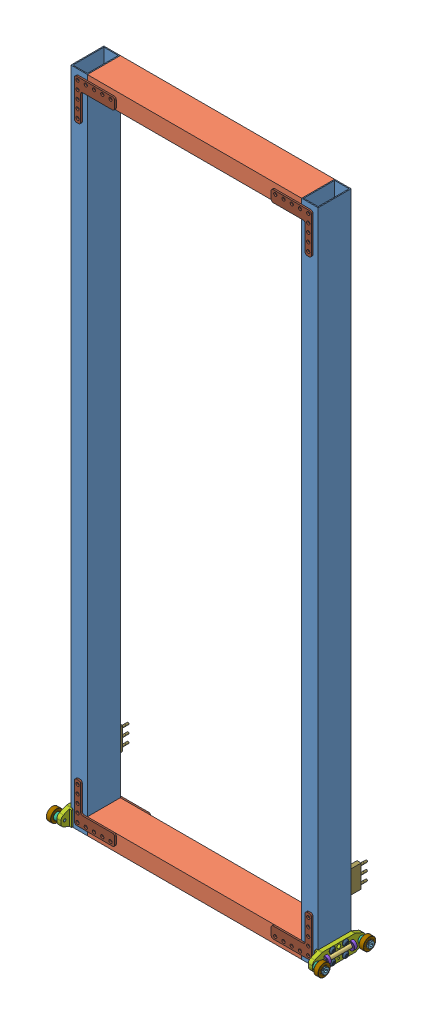
SolidWorks assembly Assem1^short elevator second stage(1), configuration Default. Lengths in mm.
Overall size (424.07 1018.01 128.54).
54 component instances, 12 part files, 44 mates.
Components (placement in the parent):
- 2x1 40in extrude-1: 2x1 40in extrude [Default] at (187.1883 1213.0001 1057.544) x (1 0 0) z (0 -1 0) size (25.4 50.8 1016)
- 2x1 40in extrude-2: 2x1 40in extrude [Default] at (542.7883 1213.0001 1057.544) x (1 0 0) z (0 -1 0) size (25.4 50.8 1016)
- 2x1 13in extrude-1: 2x1 13in extrude [Default] at (542.7883 197.0001 1108.344) x (0 0 1) z (0 -1 0) size (50.8 330.2 25.4)
- 2x1 13in extrude-2: 2x1 13in extrude [Default] at (542.7883 1187.6001 1108.344) x (0 0 1) z (0 -1 0) size (50.8 330.2 25.4)
- Bearing Block-1: Bearing Block [Default] at (-133.7189 -456.4617 -235.3019) x (-1 0 0) z (0 1 0) size (31.06 89.43 29.43)
  - Sliding Elevator Bearing Block Kit.step-1: Sliding Elevator Bearing Block Kit.step [Default] at (-2.279 1755.626 148.4607) x (0 -0.999847 -0.017493) z (-1 0 0) size (88.96 27.87 31.06)
    - .25diameter_1.75inSteelDowel_SLIDE-002.step-1: .25diameter_1.75inSteelDowel_SLIDE-002.step [Default] at (428.3334 525.2741 706.1052) x (0.999847 0.017493 0) z (0 0 1) size (44.45 6.35 6.35)
    - 10-32 Locknut 2623.step-1: 10-32 Locknut 2623.step [Default] at (418.0305 533.3501 696.4532) x (1 0 0) z (0 1 0) size (9.53 5.96 11)
    - Bearing Block Shoulder Bolt - SLIDE-004.step-1: Bearing Block Shoulder Bolt - SLIDE-004.step [Default] at (393.4137 524.6631 723.447) x (0.999978 0.006628 0) z (0 0 1) size (9.53 9.53 21.53)
    - Bearing Block Shoulder Bolt Spacer - SLIDE-003.step-1: Bearing Block Shoulder Bolt Spacer - SLIDE-003.step [Default] at (209.8469 202.8854 705.9782) x (0.999977 0.006804 0) z (0 0 1) size (10.72 10.72 5.56)
    - Sliding Bearing Block Plate - SLIDE-001.step-1: Sliding Bearing Block Plate - SLIDE-001.step [Default] at (417.8216 -325.94 699.6282) x (0.999847 0.017493 0) z (0 0 1) size (81.28 25.4 9.54)
    - TTB-0027_.50OD_.25ID_.188WD.step-1: TTB-0027_.50OD_.25ID_.188WD.step [Default] at (448.2757 525.623 706.1052) x (0 0 -1) z (0.999847 0.017493 0) size (12.7 12.7 4.76)
    - TTB-0038_75OD_25ID_28WD.step-1: TTB-0038_75OD_25ID_28WD.step [Default] at (463.253 525.885 715.1127) size (19.05 19.05 7.14)
    - Bearing Block Shoulder Bolt - SLIDE-004.step-2: Bearing Block Shoulder Bolt - SLIDE-004.step [Default] at (463.253 525.885 723.447) size (9.53 9.53 21.53)
    - TTB-0027_.50OD_.25ID_.188WD.step-2: TTB-0027_.50OD_.25ID_.188WD.step [Default] at (408.3911 524.9252 706.1052) x (0 0 -1) z (0.999847 0.017493 0) size (12.7 12.7 4.76)
    - Bearing Block Shoulder Bolt Spacer - SLIDE-003.step-2: Bearing Block Shoulder Bolt Spacer - SLIDE-003.step [Default] at (277.5012 205.3636 705.9782) size (10.72 10.72 5.56)
    - TTB-0038_75OD_25ID_28WD.step-2: TTB-0038_75OD_25ID_28WD.step [Default] at (393.4137 524.6631 715.1127) x (0.999973 0.007362 0) z (0 0 1) size (19.05 19.05 7.14)
    - .625 Long 10-32 Button Head Screw.step-1: .625 Long 10-32 Button Head Screw.step [Default] at (438.3474 533.7055 699.3234) x (0.999998 0.002032 0) z (0 0 1) size (9.17 9.17 18.44)
    - .625 Long 10-32 Button Head Screw.step-2: .625 Long 10-32 Button Head Screw.step [Default] at (438.6362 517.1981 699.3234) x (1 -0.000148 0) z (0 0 1) size (9.17 9.17 18.44)
    - .625 Long 10-32 Button Head Screw.step-3: .625 Long 10-32 Button Head Screw.step [Default] at (418.3193 516.8426 699.3234) x (0.999999 0.001159 0) z (0 0 1) size (9.17 9.17 18.44)
    - .625 Long 10-32 Button Head Screw.step-4: .625 Long 10-32 Button Head Screw.step [Default] at (418.0305 533.3501 699.3234) x (0.999983 0.005862 0) z (0 0 1) size (9.17 9.17 18.44)
    - 10-32 Locknut 2623.step-2: 10-32 Locknut 2623.step [Default] at (438.3474 533.7055 696.4532) x (0.999999 0.001134 0) z (-0.001134 0.999999 0) size (9.53 5.96 11)
    - 10-32 Locknut 2623.step-3: 10-32 Locknut 2623.step [Default] at (438.6362 517.1981 696.4532) x (1 0.000493 0) z (-0.000493 1 0) size (9.53 5.96 11)
    - 10-32 Locknut 2623.step-4: 10-32 Locknut 2623.step [Default] at (418.3193 516.8426 696.4532) x (0.999999 0.001452 0) z (-0.001452 0.999999 0) size (9.53 5.96 11)
- Copy of Copy (4) of Assem10^Assem1_short elevator second stage(1)-1: Copy of Copy (4) of Assem10^Assem1_short elevator second stage(1) [Default] at (889.0955 875.8618 -235.1495) x (1 0 0) z (0 -1 0) size (31.06 89.43 29.43) (virtual)
  - Sliding Elevator Bearing Block Kit.step-1: Sliding Elevator Bearing Block Kit.step [Default] at (-2.279 1755.626 148.4607) x (0 -0.999847 -0.017493) z (-1 0 0) size (88.96 27.87 31.06)
    - .25diameter_1.75inSteelDowel_SLIDE-002.step-1: .25diameter_1.75inSteelDowel_SLIDE-002.step [Default] at (428.3334 525.2741 706.1052) x (0.999847 0.017493 0) z (0 0 1) size (44.45 6.35 6.35)
    - 10-32 Locknut 2623.step-1: 10-32 Locknut 2623.step [Default] at (418.0305 533.3501 696.4532) x (1 0 0) z (0 1 0) size (9.53 5.96 11)
    - Bearing Block Shoulder Bolt - SLIDE-004.step-1: Bearing Block Shoulder Bolt - SLIDE-004.step [Default] at (393.4137 524.6631 723.447) x (0.999978 0.006628 0) z (0 0 1) size (9.53 9.53 21.53)
    - Bearing Block Shoulder Bolt Spacer - SLIDE-003.step-1: Bearing Block Shoulder Bolt Spacer - SLIDE-003.step [Default] at (209.8469 202.8854 705.9782) x (0.999977 0.006804 0) z (0 0 1) size (10.72 10.72 5.56)
    - Sliding Bearing Block Plate - SLIDE-001.step-1: Sliding Bearing Block Plate - SLIDE-001.step [Default] at (417.8216 -325.94 699.6282) x (0.999847 0.017493 0) z (0 0 1) size (81.28 25.4 9.54)
    - TTB-0027_.50OD_.25ID_.188WD.step-1: TTB-0027_.50OD_.25ID_.188WD.step [Default] at (448.2757 525.623 706.1052) x (0 0 -1) z (0.999847 0.017493 0) size (12.7 12.7 4.76)
    - TTB-0038_75OD_25ID_28WD.step-1: TTB-0038_75OD_25ID_28WD.step [Default] at (463.253 525.885 715.1127) size (19.05 19.05 7.14)
    - Bearing Block Shoulder Bolt - SLIDE-004.step-2: Bearing Block Shoulder Bolt - SLIDE-004.step [Default] at (463.253 525.885 723.447) size (9.53 9.53 21.53)
    - TTB-0027_.50OD_.25ID_.188WD.step-2: TTB-0027_.50OD_.25ID_.188WD.step [Default] at (408.3911 524.9252 706.1052) x (0 0 -1) z (0.999847 0.017493 0) size (12.7 12.7 4.76)
    - Bearing Block Shoulder Bolt Spacer - SLIDE-003.step-2: Bearing Block Shoulder Bolt Spacer - SLIDE-003.step [Default] at (277.5012 205.3636 705.9782) size (10.72 10.72 5.56)
    - TTB-0038_75OD_25ID_28WD.step-2: TTB-0038_75OD_25ID_28WD.step [Default] at (393.4137 524.6631 715.1127) x (0.999973 0.007362 0) z (0 0 1) size (19.05 19.05 7.14)
    - .625 Long 10-32 Button Head Screw.step-1: .625 Long 10-32 Button Head Screw.step [Default] at (438.3474 533.7055 699.3234) x (0.999998 0.002032 0) z (0 0 1) size (9.17 9.17 18.44)
    - .625 Long 10-32 Button Head Screw.step-2: .625 Long 10-32 Button Head Screw.step [Default] at (438.6362 517.1981 699.3234) x (1 -0.000148 0) z (0 0 1) size (9.17 9.17 18.44)
    - .625 Long 10-32 Button Head Screw.step-3: .625 Long 10-32 Button Head Screw.step [Default] at (418.3193 516.8426 699.3234) x (0.999999 0.001159 0) z (0 0 1) size (9.17 9.17 18.44)
    - .625 Long 10-32 Button Head Screw.step-4: .625 Long 10-32 Button Head Screw.step [Default] at (418.0305 533.3501 699.3234) x (0.999983 0.005862 0) z (0 0 1) size (9.17 9.17 18.44)
    - 10-32 Locknut 2623.step-2: 10-32 Locknut 2623.step [Default] at (438.3474 533.7055 696.4532) x (0.999999 0.001134 0) z (-0.001134 0.999999 0) size (9.53 5.96 11)
    - 10-32 Locknut 2623.step-3: 10-32 Locknut 2623.step [Default] at (438.6362 517.1981 696.4532) x (1 0.000493 0) z (-0.000493 1 0) size (9.53 5.96 11)
    - 10-32 Locknut 2623.step-4: 10-32 Locknut 2623.step [Default] at (418.3193 516.8426 696.4532) x (0.999999 0.001452 0) z (-0.001452 0.999999 0) size (9.53 5.96 11)
- L bracket thin-1: L bracket thin [Default] at (31.2018 194.4353 779.4446) x (-1 0 0) z (0 0.754511 0.656287) size (61.93 42.53 48.36)
- L bracket thin-2: L bracket thin [Default] at (31.2018 194.4353 726.1446) x (-1 0 0) z (0 0.754511 0.656287) size (61.93 42.53 48.36)
- L bracket thin-3: L bracket thin [Default] at (724.1747 194.4353 1439.7435) x (1 0 0) z (0 0.754511 -0.656287) size (61.93 42.53 48.36)
- L bracket thin-4: L bracket thin [Default] at (724.1747 194.4353 1386.4435) x (1 0 0) z (0 0.754511 -0.656287) size (61.93 42.53 48.36)
- L bracket thin-5: L bracket thin [Default] at (724.1747 1215.5648 779.4446) x (1 0 0) z (0 -0.754511 0.656287) size (61.93 42.53 48.36)
- L bracket thin-6: L bracket thin [Default] at (31.2018 1215.5648 1386.4435) x (-1 0 0) z (0 -0.754511 -0.656287) size (61.93 42.53 48.36)
- L bracket thin-7: L bracket thin [Default] at (31.2018 1215.5648 1439.7435) x (-1 0 0) z (0 -0.754511 -0.656287) size (61.93 42.53 48.36)
- L bracket thin-8: L bracket thin [Default] at (724.1747 1215.5648 726.1446) x (1 0 0) z (0 -0.754511 0.656287) size (61.93 42.53 48.36)
- chain block-1: chain block [Default] at (725.1399 192.8478 1386.4435) x (1 0 0) z (0 0.754511 -0.656287) size (13.97 43.8 43.91)
- chain block-2: chain block [Default] at (30.2366 375.7773 1386.4435) x (-1 0 0) z (0 -0.754511 -0.656287) size (13.97 43.8 43.91)
Mates (geometry in assembly coordinates):
- Coincident9: coincident anti-aligned: plane of 2x1 40in extrude-1 through (212.5883 197.0001 1057.544) normal (1 0 0); plane of 2x1 13in extrude-1 through (212.5883 197.0001 1108.344) normal (-1 0 0)
- Coincident10: coincident aligned: line of 2x1 40in extrude-1 through (212.5883 197.0001 1057.544) axis (0 0 1); line of 2x1 13in extrude-1 through (212.5883 197.0001 1057.544) axis (0 0 1)
- Coincident11: coincident aligned: line of 2x1 40in extrude-1 through (212.5883 197.0001 1108.344) axis (0 1 0); line of 2x1 13in extrude-1 through (212.5883 197.0001 1108.344) axis (0 1 0)
- Coincident14: coincident anti-aligned: plane of 2x1 40in extrude-1 through (212.5883 197.0001 1057.544) normal (1 0 0); plane of 2x1 13in extrude-2 through (212.5883 1187.6001 1108.344) normal (-1 0 0)
- Coincident15: coincident aligned: plane of 2x1 40in extrude-1 through (187.1883 197.0001 1108.344) normal (0 0 1); plane of 2x1 13in extrude-2 through (212.5883 1213.0001 1108.344) normal (0 0 1)
- Coincident16: coincident aligned: plane of 2x1 40in extrude-1 through (187.1883 1213.0001 1057.544) normal (0 1 0); plane of 2x1 13in extrude-2 through (212.5883 1213.0001 1057.544) normal (0 1 0)
- Coincident27: coincident anti-aligned: plane of 2x1 40in extrude-1 through (187.1883 197.0001 1057.544) normal (0 0 -1); plane of Copy of Copy (4) of Assem10^Assem2_short elevator(1)-1/Sliding Elevator Bearing Block Kit.step-1/Sliding Bearing Block Plate - SLIDE-001.step-1 through (187.1883 197.0001 1057.544) normal (0 0 1)
- Coincident28: coincident anti-aligned: plane of 2x1 40in extrude-1 through (187.1883 197.0001 1057.544) normal (-1 0 0); plane of Copy of Copy (4) of Assem10^Assem2_short elevator(1)-1/Sliding Elevator Bearing Block Kit.step-1/Sliding Bearing Block Plate - SLIDE-001.step-1 through (187.1883 209.7001 1083.0202) normal (1 0 0)
- Coincident29: coincident aligned: plane of 2x1 40in extrude-1 through (187.1883 197.0001 1057.544) normal (0 -1 0); plane of Copy of Copy (4) of Assem10^Assem2_short elevator(1)-1/Sliding Elevator Bearing Block Kit.step-1/Sliding Bearing Block Plate - SLIDE-001.step-1 through (187.1883 197.0001 1057.6202) normal (0 -1 0)
- Distance4: distance = 7.874 mm aligned: plane of 2x1 40in extrude-1 through (212.5883 197.0001 1057.544) normal (1 0 0); plane of L bracket thin-3 through (204.7143 222.4001 1110.844) normal (1 0 0)
- Distance5: distance = 7.874 mm aligned: plane of L bracket thin-4 through (204.7143 222.4001 1057.544) normal (1 0 0); plane of 2x1 40in extrude-1 through (212.5883 197.0001 1057.544) normal (1 0 0)
- Distance8: distance = 7.874 mm aligned: plane of L bracket thin-8 through (204.7143 1187.6001 1055.044) normal (1 0 0); plane of 2x1 40in extrude-1 through (212.5883 197.0001 1057.544) normal (1 0 0)
- Distance10: distance = 7.874 mm aligned: plane of 2x1 40in extrude-1 through (212.5883 197.0001 1057.544) normal (1 0 0); plane of L bracket thin-5 through (204.7143 1187.6001 1108.344) normal (1 0 0)
- Coincident78: coincident anti-aligned: plane of 2x1 40in extrude-1 through (187.1883 197.0001 1057.544) normal (0 0 -1); plane of chain block-1 through (198.6818 284.3126 1057.544) normal (0 0 1)
- Coincident12: coincident anti-aligned: line of 2x1 40in extrude-2 through (542.7883 197.0001 1108.344) axis (0 0 -1); line of 2x1 13in extrude-1 through (542.7883 197.0001 1057.544) axis (0 0 1)
- Coincident13: coincident aligned: plane of 2x1 40in extrude-2 through (542.7883 197.0001 1108.344) normal (0 0 1); plane of 2x1 13in extrude-1 through (212.5883 222.4001 1108.344) normal (0 0 1)
- Coincident24: coincident anti-aligned: plane of 2x1 40in extrude-2 through (568.1883 197.0001 1057.544) normal (1 0 0); plane of Copy of Copy (3) of Assem10^Assem2_short elevator(1)-1/Sliding Elevator Bearing Block Kit.step-1/Sliding Bearing Block Plate - SLIDE-001.step-1 through (568.1883 209.7001 1082.8678) normal (-1 0 0)
- Coincident25: coincident aligned: plane of 2x1 40in extrude-2 through (542.7883 197.0001 1057.544) normal (0 -1 0); plane of Copy of Copy (3) of Assem10^Assem2_short elevator(1)-1/Sliding Elevator Bearing Block Kit.step-1/Sliding Bearing Block Plate - SLIDE-001.step-1 through (568.1883 197.0001 1108.2678) normal (0 -1 0)
- Coincident26: coincident anti-aligned: plane of 2x1 40in extrude-2 through (542.7883 197.0001 1108.344) normal (0 0 1); plane of Copy of Copy (3) of Assem10^Assem2_short elevator(1)-1/Sliding Elevator Bearing Block Kit.step-1/Sliding Bearing Block Plate - SLIDE-001.step-1 through (568.1883 197.0001 1108.344) normal (0 0 -1)
- Distance3: distance = 7.874 mm aligned: plane of 2x1 40in extrude-2 through (542.7883 197.0001 1057.544) normal (-1 0 0); plane of L bracket thin-1 through (550.6623 222.4001 1108.344) normal (-1 0 0)
- Distance6: distance = 7.874 mm aligned: plane of 2x1 40in extrude-2 through (542.7883 197.0001 1057.544) normal (-1 0 0); plane of L bracket thin-2 through (550.6623 222.4001 1055.044) normal (-1 0 0)
- Distance7: distance = 7.874 mm aligned: plane of 2x1 40in extrude-2 through (542.7883 197.0001 1057.544) normal (-1 0 0); plane of L bracket thin-6 through (550.6623 1187.6001 1057.544) normal (-1 0 0)
- Distance9: distance = 7.874 mm aligned: plane of L bracket thin-7 through (550.6623 1187.6001 1110.844) normal (-1 0 0); plane of 2x1 40in extrude-2 through (542.7883 197.0001 1057.544) normal (-1 0 0)
- Coincident83: coincident anti-aligned: plane of 2x1 40in extrude-2 through (542.7883 197.0001 1057.544) normal (0 0 -1); plane of chain block-2 through (556.6948 284.3126 1057.544) normal (0 0 1)
- Coincident45: coincident anti-aligned: plane of 2x1 13in extrude-1 through (212.5883 222.4001 1108.344) normal (0 0 1); plane of L bracket thin-1 through (529.2501 235.8875 1108.344) normal (0 0 -1)
- Coincident47: coincident aligned: plane of 2x1 13in extrude-1 through (212.5883 222.4001 1057.544) normal (0 1 0); plane of L bracket thin-1 through (498.2875 222.4001 1110.844) normal (0 1 0)
- Coincident50: coincident anti-aligned: plane of 2x1 13in extrude-1 through (212.5883 222.4001 1108.344) normal (0 0 1); plane of L bracket thin-3 through (226.1265 235.8875 1108.344) normal (0 0 -1)
- Coincident51: coincident aligned: plane of 2x1 13in extrude-1 through (212.5883 222.4001 1057.544) normal (0 1 0); plane of L bracket thin-3 through (257.0891 222.4001 1108.344) normal (0 1 0)
- Coincident53: coincident anti-aligned: plane of 2x1 13in extrude-1 through (212.5883 222.4001 1057.544) normal (0 0 -1); plane of L bracket thin-4 through (226.1265 235.8875 1057.544) normal (0 0 1)
- Coincident55: coincident aligned: plane of 2x1 13in extrude-1 through (212.5883 222.4001 1057.544) normal (0 1 0); plane of L bracket thin-4 through (257.0891 222.4001 1055.044) normal (0 1 0)
- Coincident57: coincident anti-aligned: plane of 2x1 13in extrude-1 through (212.5883 222.4001 1057.544) normal (0 0 -1); plane of L bracket thin-2 through (529.2501 235.8875 1057.544) normal (0 0 1)
- Coincident58: coincident aligned: plane of 2x1 13in extrude-1 through (212.5883 222.4001 1057.544) normal (0 1 0); plane of L bracket thin-2 through (498.2875 222.4001 1057.544) normal (0 1 0)
- Coincident60: coincident anti-aligned: plane of 2x1 13in extrude-2 through (212.5883 1213.0001 1057.544) normal (0 0 -1); plane of L bracket thin-6 through (529.2501 1174.1127 1057.544) normal (0 0 1)
- Coincident61: coincident aligned: plane of 2x1 13in extrude-2 through (212.5883 1187.6001 1057.544) normal (0 -1 0); plane of L bracket thin-6 through (498.2875 1187.6001 1055.044) normal (0 -1 0)
- Coincident63: coincident anti-aligned: plane of 2x1 13in extrude-2 through (212.5883 1213.0001 1057.544) normal (0 0 -1); plane of L bracket thin-8 through (226.1265 1174.1127 1057.544) normal (0 0 1)
- Coincident64: coincident: plane of 2x1 13in extrude-2 through (212.5883 1187.6001 1057.544) normal (0 -1 0); line of L bracket thin-8 through (253.9141 1187.6001 1055.044) axis (-1 0 0)
- Coincident66: coincident anti-aligned: plane of 2x1 13in extrude-2 through (212.5883 1213.0001 1108.344) normal (0 0 1); plane of L bracket thin-7 through (529.2501 1174.1127 1108.344) normal (0 0 -1)
- Coincident67: coincident aligned: plane of 2x1 13in extrude-2 through (212.5883 1187.6001 1057.544) normal (0 -1 0); plane of L bracket thin-7 through (498.2875 1187.6001 1108.344) normal (0 -1 0)
- Coincident69: coincident anti-aligned: plane of 2x1 13in extrude-2 through (212.5883 1213.0001 1108.344) normal (0 0 1); plane of L bracket thin-5 through (226.1265 1174.1127 1108.344) normal (0 0 -1)
- Coincident70: coincident aligned: plane of 2x1 13in extrude-2 through (212.5883 1187.6001 1057.544) normal (0 -1 0); plane of L bracket thin-5 through (257.0891 1187.6001 1110.844) normal (0 -1 0)
- Coincident84: coincident aligned: plane of L bracket thin-2 through (550.6623 222.4001 1055.044) normal (-1 0 0); plane of chain block-2 through (550.6623 266.8501 1052.7688) normal (-1 0 0)
- Coincident85: coincident anti-aligned: plane of L bracket thin-2 through (542.7375 266.8501 1057.544) normal (0 1 0); plane of chain block-2 through (564.6323 266.8501 1057.544) normal (0 -1 0)
- Coincident81: coincident aligned: plane of L bracket thin-4 through (204.7143 222.4001 1057.544) normal (1 0 0); plane of chain block-1 through (204.7143 301.7751 1052.7688) normal (1 0 0)
- Coincident82: coincident anti-aligned: plane of L bracket thin-4 through (212.6391 266.8501 1055.044) normal (0 1 0); plane of chain block-1 through (206.6193 266.8501 1057.544) normal (0 -1 0)
